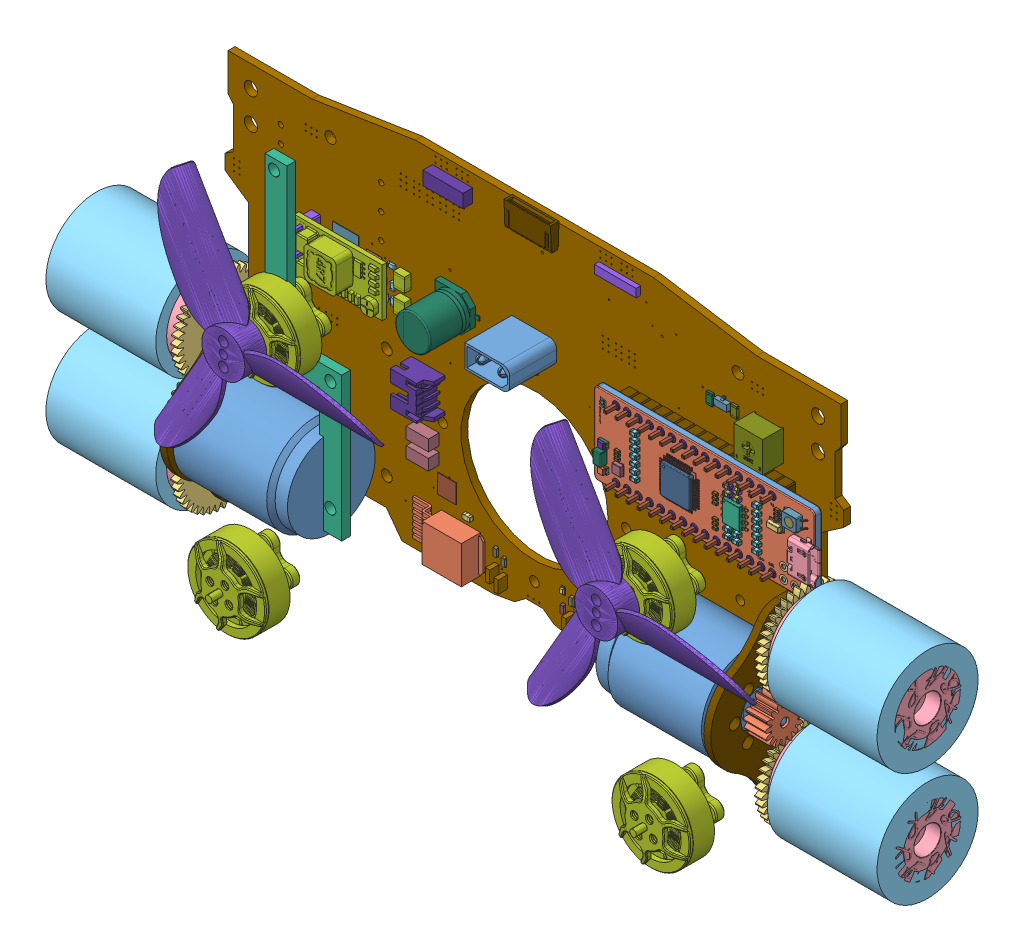
SolidWorks assembly Ensamblaje60, configuration Predeterminado. Lengths in mm.
Overall size (189.47 95.17 43.77).
248 component instances, 80 part files, 7 mates.
Components (placement in the parent):
- placa v11-1: placa v11 [Predeterminado] at (-59.8696 -16.4339 -3.9696) size (140.86 80.97 16.6)
  - placa v11.step-1: placa v11.step [Predeterminado] at origin size (140.86 80.97 16.6)
    - PCB Component.step-1: PCB Component.step [Predeterminado] at origin size (140.86 80.97 16.6)
      - LED-0603 (1).step-1: LED-0603 (1).step [Predeterminado] at (70.275 8.61 1.57) x (0 -1 0) z (0 0 1) size (1.61 0.81 0.61)
        - Pocket002.step-1: Pocket002.step [Predeterminado] at origin size (0.41 0.81 0.21)
        - Pad004.step-1: Pad004.step [Predeterminado] x (1 0 0) z (0 0 -1) size (0.4 0.8 0)
        - Fillet.step-1: Fillet.step [Predeterminado] at origin size (1 0.7 0.4)
        - Pocket001.step-1: Pocket001.step [Predeterminado] at origin size (0.4 0.8 0.2)
        - Pad.step-1: Pad.step [Predeterminado] at origin size (0.8 0.8 0.2)
      - ARDUINO-NANO-3.0.step-1: ARDUINO-NANO-3.0.step [Predeterminado] at (104.204 47.47 1.57) size (51.66 18.54 11.82)
        - 1.step.step-1: 1.step.step [Predeterminado] at (9.2423 0.0433 4.14) x (0 -1 0) z (0 0 1) size (4.9 6 1)
          - 1-0.step.step-1: 1-0.step.step [Predeterminado] at (0 0 0.08) size (4.9 3.9 0.92)
          - 2.step.step-1: 2.step.step [Predeterminado] at (0.635 0 0) size (4.23 6 0.62)
          - Name1.step.step-1: Name1.step.step [Predeterminado] at (-0.0045 -0.5756 0.3787) x (-1 0 0) z (0 1 0) size (0.25 0.13 0.25)
          - thermal pad.step.step-1: thermal pad.step.step [Predeterminado] at (0 0 0.08) x (-1 0 0) z (0 0 -1) size (3.2 2.4 0.1)
        - QFP Template.step.step-1: QFP Template.step.step [Predeterminado] at (-3.3256 -0.4727 4.14) x (0 -1 0) z (0 0 1) size (9 9 1.2)
          - Body.step.step-1: Body.step.step [Predeterminado] at (0 0 0.15) size (7 7 1.05)
          - Leg.step.step-1: Leg.step.step [Predeterminado] at (0 0.25 0) x (1 0 0) z (0 -1 0) size (9 0.75 5.72)
          - Leg.step.step-2: Leg.step.step [Predeterminado] at (-0.25 0 0) x (0 1 0) z (1 0 0) size (9 0.75 5.72)
          - name2.step.step-1: name2.step.step [Predeterminado] at (1.2257 1.5908 1.101) size (0.47 0.47 0.1)
        - QFP Template.step (1).step-1: QFP Template.step (1).step [Predeterminado] at (11.7079 0.2587 2.54) x (0 -1 0) z (0 0 -1) size (9 9 1.2)
          - Body.step.step-1: Body.step.step [Predeterminado] at (0 0 0.15) size (7 7 1.05)
          - Leg.step.step-1: Leg.step.step [Predeterminado] at (0 0.25 0) x (1 0 0) z (0 -1 0) size (9 0.75 5.72)
          - Leg.step.step-2: Leg.step.step [Predeterminado] at (-0.25 0 0) x (0 1 0) z (1 0 0) size (9 0.75 5.72)
          - name2.step.step-1: name2.step.step [Predeterminado] at (1.2257 1.5908 1.101) size (0.47 0.47 0.1)
        - 1-1.step.step-1: 1-1.step.step [Predeterminado] at (-17.0798 -4.3486 4.14) size (2 2 0.8)
          - 1-2.step.step-1: 1-2.step.step [Predeterminado] at (0 0 0.02) size (2 2 0.78)
          - 2-3.step.step-1: 2-3.step.step [Predeterminado] at origin size (2 1.6 0.2)
        - 1-2-4.step.step-1: 1-2-4.step.step [Predeterminado] at (-20.4345 -1.0096 4.14) size (2 1.25 1.09)
          - 1-5.step.step-1: 1-5.step.step [Predeterminado] at (0 0 0.01) size (1.98 1.25 0.58)
          - 2-6.step.step-1: 2-6.step.step [Predeterminado] at (0.001 0 0) size (2 1.25 0.6)
          - 3.step.step-1: 3.step.step [Predeterminado] at (0.001 0 0.59) x (-1 0 0) z (0 0 1) size (1.45 1.25 0.5)
        - 1-3.step.step-1: 1-3.step.step [Predeterminado] at (-20.4345 -6.0538 4.14) size (2 1.25 1.09)
          - 1-7.step.step-1: 1-7.step.step [Predeterminado] at (0 0 0.01) size (1.98 1.25 0.58)
          - 2-8.step.step-1: 2-8.step.step [Predeterminado] at (0.001 0 0) size (2 1.25 0.6)
          - 3-9.step.step-1: 3-9.step.step [Predeterminado] at (0.001 0 0.59) x (-1 0 0) z (0 0 1) size (1.45 1.25 0.5)
        - 1-4.step.step-1: 1-4.step.step [Predeterminado] at (18.758 2.4348 4.14) x (0 -1 0) z (0 0 1) size (2.3 2.86 1.1)
          - 1-10.step.step-1: 1-10.step.step [Predeterminado] at (0 0 0.055) size (1.3 2.86 1.04)
          - 2-11.step.step-1: 2-11.step.step [Predeterminado] x (1 0 0) z (0 -1 0) size (2.3 0.55 2.35)
        - 3-12.step.step-1: 3-12.step.step [Predeterminado] at (14.649 -4.6077 5.09) x (-1 0 0) z (0 0 -1) size (1.6 0.8 0.95)
          - 1-13.step.step-1: 1-13.step.step [Predeterminado] at (-0.78 0.38 0.93) x (1 0 0) z (0 0 -1) size (1.56 0.76 0.91)
          - 2-14.step.step-1: 2-14.step.step [Predeterminado] at (0 0 0.95) x (1 0 0) z (0 0 -1) size (1.6 0.8 0.95)
        - 3-12.step (1).step-1: 3-12.step (1).step [Predeterminado] at (-13.1027 -4.224 5.09) x (-1 0 0) z (0 0 -1) size (1.6 0.8 0.95)
          - 1-13.step.step-1: 1-13.step.step [Predeterminado] at (-0.78 0.38 0.93) x (1 0 0) z (0 0 -1) size (1.56 0.76 0.91)
          - 2-14.step.step-1: 2-14.step.step [Predeterminado] at (0 0 0.95) x (1 0 0) z (0 0 -1) size (1.6 0.8 0.95)
        - 3-12.step (2).step-1: 3-12.step (2).step [Predeterminado] at (14.649 -3.1077 5.09) x (-1 0 0) z (0 0 -1) size (1.6 0.8 0.95)
          - 1-13.step.step-1: 1-13.step.step [Predeterminado] at (-0.78 0.38 0.93) x (1 0 0) z (0 0 -1) size (1.56 0.76 0.91)
          - 2-14.step.step-1: 2-14.step.step [Predeterminado] at (0 0 0.95) x (1 0 0) z (0 0 -1) size (1.6 0.8 0.95)
        - 3-12.step (3).step-1: 3-12.step (3).step [Predeterminado] at (-13.1027 -2.724 5.09) x (-1 0 0) z (0 0 -1) size (1.6 0.8 0.95)
          - 1-13.step.step-1: 1-13.step.step [Predeterminado] at (-0.78 0.38 0.93) x (1 0 0) z (0 0 -1) size (1.56 0.76 0.91)
          - 2-14.step.step-1: 2-14.step.step [Predeterminado] at (0 0 0.95) x (1 0 0) z (0 0 -1) size (1.6 0.8 0.95)
        - 3-12.step (4).step-1: 3-12.step (4).step [Predeterminado] at (14.649 -1.6077 5.09) x (-1 0 0) z (0 0 -1) size (1.6 0.8 0.95)
          - 1-13.step.step-1: 1-13.step.step [Predeterminado] at (-0.78 0.38 0.93) x (1 0 0) z (0 0 -1) size (1.56 0.76 0.91)
          - 2-14.step.step-1: 2-14.step.step [Predeterminado] at (0 0 0.95) x (1 0 0) z (0 0 -1) size (1.6 0.8 0.95)
        - 3-12.step (5).step-1: 3-12.step (5).step [Predeterminado] at (-13.1027 -1.224 5.09) x (-1 0 0) z (0 0 -1) size (1.6 0.8 0.95)
          - 1-13.step.step-1: 1-13.step.step [Predeterminado] at (-0.78 0.38 0.93) x (1 0 0) z (0 0 -1) size (1.56 0.76 0.91)
          - 2-14.step.step-1: 2-14.step.step [Predeterminado] at (0 0 0.95) x (1 0 0) z (0 0 -1) size (1.6 0.8 0.95)
        - 3-12.step (6).step-1: 3-12.step (6).step [Predeterminado] at (14.649 -0.1077 5.09) x (-1 0 0) z (0 0 -1) size (1.6 0.8 0.95)
          - 1-13.step.step-1: 1-13.step.step [Predeterminado] at (-0.78 0.38 0.93) x (1 0 0) z (0 0 -1) size (1.56 0.76 0.91)
          - 2-14.step.step-1: 2-14.step.step [Predeterminado] at (0 0 0.95) x (1 0 0) z (0 0 -1) size (1.6 0.8 0.95)
        - 3-12.step (7).step-1: 3-12.step (7).step [Predeterminado] at (-13.1027 0.276 5.09) x (-1 0 0) z (0 0 -1) size (1.6 0.8 0.95)
          - 1-13.step.step-1: 1-13.step.step [Predeterminado] at (-0.78 0.38 0.93) x (1 0 0) z (0 0 -1) size (1.56 0.76 0.91)
          - 2-14.step.step-1: 2-14.step.step [Predeterminado] at (0 0 0.95) x (1 0 0) z (0 0 -1) size (1.6 0.8 0.95)
        - 3-12.step (8).step-1: 3-12.step (8).step [Predeterminado] at (14.649 1.3923 5.09) x (-1 0 0) z (0 0 -1) size (1.6 0.8 0.95)
          - 1-13.step.step-1: 1-13.step.step [Predeterminado] at (-0.78 0.38 0.93) x (1 0 0) z (0 0 -1) size (1.56 0.76 0.91)
          - 2-14.step.step-1: 2-14.step.step [Predeterminado] at (0 0 0.95) x (1 0 0) z (0 0 -1) size (1.6 0.8 0.95)
        - 3-12.step (9).step-1: 3-12.step (9).step [Predeterminado] at (-13.1027 1.776 5.09) x (-1 0 0) z (0 0 -1) size (1.6 0.8 0.95)
          - 1-13.step.step-1: 1-13.step.step [Predeterminado] at (-0.78 0.38 0.93) x (1 0 0) z (0 0 -1) size (1.56 0.76 0.91)
          - 2-14.step.step-1: 2-14.step.step [Predeterminado] at (0 0 0.95) x (1 0 0) z (0 0 -1) size (1.6 0.8 0.95)
        - 3-12.step (10).step-1: 3-12.step (10).step [Predeterminado] at (14.649 2.8923 5.09) x (-1 0 0) z (0 0 -1) size (1.6 0.8 0.95)
          - 1-13.step.step-1: 1-13.step.step [Predeterminado] at (-0.78 0.38 0.93) x (1 0 0) z (0 0 -1) size (1.56 0.76 0.91)
          - 2-14.step.step-1: 2-14.step.step [Predeterminado] at (0 0 0.95) x (1 0 0) z (0 0 -1) size (1.6 0.8 0.95)
        - 3-12.step (11).step-1: 3-12.step (11).step [Predeterminado] at (-13.1027 3.276 5.09) x (-1 0 0) z (0 0 -1) size (1.6 0.8 0.95)
          - 1-13.step.step-1: 1-13.step.step [Predeterminado] at (-0.78 0.38 0.93) x (1 0 0) z (0 0 -1) size (1.56 0.76 0.91)
          - 2-14.step.step-1: 2-14.step.step [Predeterminado] at (0 0 0.95) x (1 0 0) z (0 0 -1) size (1.6 0.8 0.95)
        - 3-12.step (12).step-1: 3-12.step (12).step [Predeterminado] at (14.649 4.3923 5.09) x (-1 0 0) z (0 0 -1) size (1.6 0.8 0.95)
          - 1-13.step.step-1: 1-13.step.step [Predeterminado] at (-0.78 0.38 0.93) x (1 0 0) z (0 0 -1) size (1.56 0.76 0.91)
          - 2-14.step.step-1: 2-14.step.step [Predeterminado] at (0 0 0.95) x (1 0 0) z (0 0 -1) size (1.6 0.8 0.95)
        - 3-12.step (13).step-1: 3-12.step (13).step [Predeterminado] at (-13.1027 4.776 5.09) x (-1 0 0) z (0 0 -1) size (1.6 0.8 0.95)
          - 1-13.step.step-1: 1-13.step.step [Predeterminado] at (-0.78 0.38 0.93) x (1 0 0) z (0 0 -1) size (1.56 0.76 0.91)
          - 2-14.step.step-1: 2-14.step.step [Predeterminado] at (0 0 0.95) x (1 0 0) z (0 0 -1) size (1.6 0.8 0.95)
        - 3-12.step (14).step-1: 3-12.step (14).step [Predeterminado] at (10.1169 -4.9732 4.14) size (1.6 0.8 0.95)
          - 1-13.step.step-1: 1-13.step.step [Predeterminado] at (-0.78 0.38 0.93) x (1 0 0) z (0 0 -1) size (1.56 0.76 0.91)
          - 2-14.step.step-1: 2-14.step.step [Predeterminado] at (0 0 0.95) x (1 0 0) z (0 0 -1) size (1.6 0.8 0.95)
        - 3-12.step (15).step-1: 3-12.step (15).step [Predeterminado] at (8.1169 -4.9732 4.14) size (1.6 0.8 0.95)
          - 1-13.step.step-1: 1-13.step.step [Predeterminado] at (-0.78 0.38 0.93) x (1 0 0) z (0 0 -1) size (1.56 0.76 0.91)
          - 2-14.step.step-1: 2-14.step.step [Predeterminado] at (0 0 0.95) x (1 0 0) z (0 0 -1) size (1.6 0.8 0.95)
        - 3-12.step (16).step-1: 3-12.step (16).step [Predeterminado] at (10.1169 -3.4732 4.14) size (1.6 0.8 0.95)
          - 1-13.step.step-1: 1-13.step.step [Predeterminado] at (-0.78 0.38 0.93) x (1 0 0) z (0 0 -1) size (1.56 0.76 0.91)
          - 2-14.step.step-1: 2-14.step.step [Predeterminado] at (0 0 0.95) x (1 0 0) z (0 0 -1) size (1.6 0.8 0.95)
        - 3-12.step (17).step-1: 3-12.step (17).step [Predeterminado] at (8.1169 -3.4732 4.14) size (1.6 0.8 0.95)
          - 1-13.step.step-1: 1-13.step.step [Predeterminado] at (-0.78 0.38 0.93) x (1 0 0) z (0 0 -1) size (1.56 0.76 0.91)
          - 2-14.step.step-1: 2-14.step.step [Predeterminado] at (0 0 0.95) x (1 0 0) z (0 0 -1) size (1.6 0.8 0.95)
        - 3_MIR.step.step-1: 3_MIR.step.step [Predeterminado] at (10.1169 4.9732 4.14) x (1 0 0) z (0 0 -1) size (1.6 0.8 0.95)
          - 1_MIR.step.step-1: 1_MIR.step.step [Predeterminado] at (-0.78 0.38 -0.93) x (1 0 0) z (0 0 -1) size (1.56 0.76 0.91)
          - 2_MIR.step.step-1: 2_MIR.step.step [Predeterminado] at (0 0 -0.95) x (1 0 0) z (0 0 -1) size (1.6 0.8 0.95)
        - 3_MIR.step (1).step-1: 3_MIR.step (1).step [Predeterminado] at (8.1169 4.9732 4.14) x (1 0 0) z (0 0 -1) size (1.6 0.8 0.95)
          - 1_MIR.step.step-1: 1_MIR.step.step [Predeterminado] at (-0.78 0.38 -0.93) x (1 0 0) z (0 0 -1) size (1.56 0.76 0.91)
          - 2_MIR.step.step-1: 2_MIR.step.step [Predeterminado] at (0 0 -0.95) x (1 0 0) z (0 0 -1) size (1.6 0.8 0.95)
        - 3_MIR.step (2).step-1: 3_MIR.step (2).step [Predeterminado] at (10.1169 3.4732 4.14) x (1 0 0) z (0 0 -1) size (1.6 0.8 0.95)
          - 1_MIR.step.step-1: 1_MIR.step.step [Predeterminado] at (-0.78 0.38 -0.93) x (1 0 0) z (0 0 -1) size (1.56 0.76 0.91)
          - 2_MIR.step.step-1: 2_MIR.step.step [Predeterminado] at (0 0 -0.95) x (1 0 0) z (0 0 -1) size (1.6 0.8 0.95)
        - 3_MIR.step (3).step-1: 3_MIR.step (3).step [Predeterminado] at (8.1169 3.4732 4.14) x (1 0 0) z (0 0 -1) size (1.6 0.8 0.95)
          - 1_MIR.step.step-1: 1_MIR.step.step [Predeterminado] at (-0.78 0.38 -0.93) x (1 0 0) z (0 0 -1) size (1.56 0.76 0.91)
          - 2_MIR.step.step-1: 2_MIR.step.step [Predeterminado] at (0 0 -0.95) x (1 0 0) z (0 0 -1) size (1.6 0.8 0.95)
        - 3-1.step.step-1: 3-1.step.step [Predeterminado] at (19.0751 5.5632 4.69) x (-1 0 0) z (0 0 -1) size (1 0.5 0.55)
          - 1-15.step.step-1: 1-15.step.step [Predeterminado] at (-0.49 0.24 0.54) x (1 0 0) z (0 0 -1) size (0.98 0.48 0.53)
          - 2-16.step.step-1: 2-16.step.step [Predeterminado] at (-0.5 0.25 0.55) x (1 0 0) z (0 0 -1) size (1 0.5 0.55)
        - 3-1.step (1).step-1: 3-1.step (1).step [Predeterminado] at (19.0751 4.7491 4.69) x (-1 0 0) z (0 0 -1) size (1 0.5 0.55)
          - 1-15.step.step-1: 1-15.step.step [Predeterminado] at (-0.49 0.24 0.54) x (1 0 0) z (0 0 -1) size (0.98 0.48 0.53)
          - 2-16.step.step-1: 2-16.step.step [Predeterminado] at (-0.5 0.25 0.55) x (1 0 0) z (0 0 -1) size (1 0.5 0.55)
        - 3-1.step (2).step-1: 3-1.step (2).step [Predeterminado] at (19.0751 3.9392 4.69) x (-1 0 0) z (0 0 -1) size (1 0.5 0.55)
          - 1-15.step.step-1: 1-15.step.step [Predeterminado] at (-0.49 0.24 0.54) x (1 0 0) z (0 0 -1) size (0.98 0.48 0.53)
          - 2-16.step.step-1: 2-16.step.step [Predeterminado] at (-0.5 0.25 0.55) x (1 0 0) z (0 0 -1) size (1 0.5 0.55)
        - 3-1.step (3).step-1: 3-1.step (3).step [Predeterminado] at (-17.3312 -0.9835 4.69) x (-1 0 0) z (0 0 -1) size (1 0.5 0.55)
          - 1-15.step.step-1: 1-15.step.step [Predeterminado] at (-0.49 0.24 0.54) x (1 0 0) z (0 0 -1) size (0.98 0.48 0.53)
          - 2-16.step.step-1: 2-16.step.step [Predeterminado] at (-0.5 0.25 0.55) x (1 0 0) z (0 0 -1) size (1 0.5 0.55)
        - 3-1.step (4).step-1: 3-1.step (4).step [Predeterminado] at (-17.3312 -2.5605 4.69) x (-1 0 0) z (0 0 -1) size (1 0.5 0.55)
          - 1-15.step.step-1: 1-15.step.step [Predeterminado] at (-0.49 0.24 0.54) x (1 0 0) z (0 0 -1) size (0.98 0.48 0.53)
          - 2-16.step.step-1: 2-16.step.step [Predeterminado] at (-0.5 0.25 0.55) x (1 0 0) z (0 0 -1) size (1 0.5 0.55)
        - 3-1.step (5).step-1: 3-1.step (5).step [Predeterminado] at (-17.3312 -1.7295 4.69) x (-1 0 0) z (0 0 -1) size (1 0.5 0.55)
          - 1-15.step.step-1: 1-15.step.step [Predeterminado] at (-0.49 0.24 0.54) x (1 0 0) z (0 0 -1) size (0.98 0.48 0.53)
          - 2-16.step.step-1: 2-16.step.step [Predeterminado] at (-0.5 0.25 0.55) x (1 0 0) z (0 0 -1) size (1 0.5 0.55)
        - 3-1.step (6).step-1: 3-1.step (6).step [Predeterminado] at (5.0242 -5.0165 4.69) x (-1 0 0) z (0 0 -1) size (1 0.5 0.55)
          - 1-15.step.step-1: 1-15.step.step [Predeterminado] at (-0.49 0.24 0.54) x (1 0 0) z (0 0 -1) size (0.98 0.48 0.53)
          - 2-16.step.step-1: 2-16.step.step [Predeterminado] at (-0.5 0.25 0.55) x (1 0 0) z (0 0 -1) size (1 0.5 0.55)
        - 3-1.step (7).step-1: 3-1.step (7).step [Predeterminado] at (5.0242 -4.0978 4.69) x (-1 0 0) z (0 0 -1) size (1 0.5 0.55)
          - 1-15.step.step-1: 1-15.step.step [Predeterminado] at (-0.49 0.24 0.54) x (1 0 0) z (0 0 -1) size (0.98 0.48 0.53)
          - 2-16.step.step-1: 2-16.step.step [Predeterminado] at (-0.5 0.25 0.55) x (1 0 0) z (0 0 -1) size (1 0.5 0.55)
        - 3-1.step (8).step-1: 3-1.step (8).step [Predeterminado] at (5.0242 -3.2174 4.69) x (-1 0 0) z (0 0 -1) size (1 0.5 0.55)
          - 1-15.step.step-1: 1-15.step.step [Predeterminado] at (-0.49 0.24 0.54) x (1 0 0) z (0 0 -1) size (0.98 0.48 0.53)
          - 2-16.step.step-1: 2-16.step.step [Predeterminado] at (-0.5 0.25 0.55) x (1 0 0) z (0 0 -1) size (1 0.5 0.55)
        - 3-1.step (9).step-1: 3-1.step (9).step [Predeterminado] at (5.0242 -0.0165 4.69) x (-1 0 0) z (0 0 -1) size (1 0.5 0.55)
          - 1-15.step.step-1: 1-15.step.step [Predeterminado] at (-0.49 0.24 0.54) x (1 0 0) z (0 0 -1) size (0.98 0.48 0.53)
          - 2-16.step.step-1: 2-16.step.step [Predeterminado] at (-0.5 0.25 0.55) x (1 0 0) z (0 0 -1) size (1 0.5 0.55)
        - 3-1.step (10).step-1: 3-1.step (10).step [Predeterminado] at (5.0242 0.9022 4.69) x (-1 0 0) z (0 0 -1) size (1 0.5 0.55)
          - 1-15.step.step-1: 1-15.step.step [Predeterminado] at (-0.49 0.24 0.54) x (1 0 0) z (0 0 -1) size (0.98 0.48 0.53)
          - 2-16.step.step-1: 2-16.step.step [Predeterminado] at (-0.5 0.25 0.55) x (1 0 0) z (0 0 -1) size (1 0.5 0.55)
        - 3-1.step (11).step-1: 3-1.step (11).step [Predeterminado] at (5.0242 1.7826 4.69) x (-1 0 0) z (0 0 -1) size (1 0.5 0.55)
          - 1-15.step.step-1: 1-15.step.step [Predeterminado] at (-0.49 0.24 0.54) x (1 0 0) z (0 0 -1) size (0.98 0.48 0.53)
          - 2-16.step.step-1: 2-16.step.step [Predeterminado] at (-0.5 0.25 0.55) x (1 0 0) z (0 0 -1) size (1 0.5 0.55)
        - 1-17.step.step-1: 1-17.step.step [Predeterminado] at (2.2426 0 2.54) x (0 -1 0) z (0 0 1) size (15.88 36.2 11.76)
        - 2-18.step.step-1: 2-18.step.step [Predeterminado] at (2.2426 0 2.54) x (0 -1 0) z (0 0 1) size (1.95 1.95 0.2)
        - 3-19.step.step-1: 3-19.step.step [Predeterminado] at (2.2426 0 2.54) x (0 -1 0) z (0 0 1) size (1.8 5.28 0.86)
        - 4.step.step-1: 4.step.step [Predeterminado] at (2.2426 0 2.54) x (0 -1 0) z (0 0 1) size (2.98 3.39 1.49)
        - 6.step.step-1: 6.step.step [Predeterminado] at (2.2426 0 2.54) x (0 -1 0) z (0 0 1) size (2.83 1.84 1.5)
        - 7.step.step-1: 7.step.step [Predeterminado] at (2.2426 0 2.54) x (0 -1 0) z (0 0 1) size (0.97 0.6 0.51)
        - 8.step.step-1: 8.step.step [Predeterminado] at (2.2426 0 2.54) x (0 -1 0) z (0 0 1) size (16.96 37.28 0.1)
        - 9.step.step-1: 9.step.step [Predeterminado] at (2.2426 0 2.54) x (0 -1 0) z (0 0 1) size (17.78 38.1 2.54)
        - 10.step.step-1: 10.step.step [Predeterminado] at (2.2426 0 2.54) x (0 -1 0) z (0 0 1) size (18.54 50.29 1.2)
        - 11.step.step-1: 11.step.step [Predeterminado] at (2.2426 0 2.54) x (0 -1 0) z (0 0 1) size (18.54 50.29 1.6)
        - 12.step.step-1: 12.step.step [Predeterminado] at (2.2426 0 2.54) x (0 -1 0) z (0 0 1) size (4.34 6.88 1.6)
        - USB Connector.step.step-1: USB Connector.step.step [Predeterminado] at (26.0074 -0.1867 5.365) x (0 1 0) z (1 0 0) size (8.2 3.3 5.4)
        - 13.step.step-1: 13.step.step [Predeterminado] at (2.2426 0 4.14) x (0 -1 0) z (0 0 1) size (12.46 38.74 0)
        - STM Logo.step.step-1: STM Logo.step.step [Predeterminado] at (-19.8495 -2.5718 4.041) x (0 -1 0) z (0 0 1) size (5.5 1.52 0.1)
      - HW-613.step-1: HW-613.step [Predeterminado] at (12.49 44.591 1.57) size (20 11 13.1)
        - 05KJ_Mini_PCB_Regulator.step-1: 05KJ_Mini_PCB_Regulator.step [Predeterminado] at (19.8629 10.8309 2.3992) x (0 -1 0) z (-1 0 0) size (11 4.81 20)
        - 1_Male_Pin_2.54_mm.step-1: 1_Male_Pin_2.54_mm.step [Predeterminado] at (1.6879 8.8159 5.3992) x (0 1 0) z (-1 0 0) size (2.54 11.1 2.4)
        - 1_Male_Pin_2.54_mm.step-2: 1_Male_Pin_2.54_mm.step [Predeterminado] at (1.6879 6.2759 5.3992) x (0 1 0) z (-1 0 0) size (2.54 11.1 2.4)
        - 1_Male_Pin_2.54_mm.step-3: 1_Male_Pin_2.54_mm.step [Predeterminado] at (1.6879 3.7359 5.3992) x (0 1 0) z (-1 0 0) size (2.54 11.1 2.4)
        - 1_Male_Pin_2.54_mm.step-4: 1_Male_Pin_2.54_mm.step [Predeterminado] at (1.6879 1.1959 5.3992) x (0 1 0) z (-1 0 0) size (2.54 11.1 2.4)
      - Board.step-1: Board.step [Predeterminado] at origin size (140.86 80.59 1.57)
      - MOMENTARY-SWITCH-SPST-SMD-5.2-REDUNDANT.step-1: MOMENTARY-SWITCH-SPST-SMD-5.2-REDUNDANT.step [Predeterminado] at (7.486 44.336 1.57) size (6.4 5.3 1.5)
      - 10k_2.step-1: 10k_2.step [Predeterminado] at (7.386 40.707 1.57) size (2.5 1.4 0.5)
      - LED-0603.step-1: LED-0603.step [Predeterminado] at (55.035 8.61 1.57) x (0 -1 0) z (0 0 1) size (2.1 0.8 0.6)
      - 10k.step-1: 10k.step [Predeterminado] at (70.312 4.989 1.57) x (0 -1 0) z (0 0 1) size (2.1 0.8 0.6)
      - 2N7002CK.step-1: 2N7002CK.step [Predeterminado] at (106.952 63.962 1.57) size (3 2.5 1.1)
      - 103.step-1: 103.step [Predeterminado] at (103.896 63.305 1.57) x (0 -1 0) z (0 0 1) size (2.5 1.4 0.5)
      - 10k_1.step-1: 10k_1.step [Predeterminado] at (109.485 63.628 1.57) x (0 -1 0) z (0 0 1) size (2.5 1.4 0.5)
      - JST-XH-03-PIN-LONG-PAD.step-1: JST-XH-03-PIN-LONG-PAD.step [Predeterminado] at (39.428 34.17 1.57) x (0 -1 0) z (0 0 1) size (7.9 7.6 8.2)
      - FH12-08S-1SH.step-1: FH12-08S-1SH.step [Predeterminado] at (63.91 77.561 1.57) x (-1 0 0) z (0 0 1) size (10.6 6.5 1.92)
      - 10k_2.step-2: 10k_2.step [Predeterminado] at (7.262 48.989 1.57) size (2.5 1.4 0.5)
      - LED-0603.step-2: LED-0603.step [Predeterminado] at (56.895 7.53 1.57) x (0 -1 0) z (0 0 1) size (2.1 0.8 0.6)
      - LED-0603.step-3: LED-0603.step [Predeterminado] at (72.322 7.486 1.57) x (0 -1 0) z (0 0 1) size (2.1 0.8 0.6)
      - XT30UPB-M.step-1: XT30UPB-M.step [Predeterminado] at (63.686 54.256 1.57) x (-1 0 0) z (0 0 1) size (10.2 5.25 13.7)
      - TLE5206-2G.step-1: TLE5206-2G.step [Predeterminado] at (44.309 6.214 1.57) x (0 -1 0) z (0 0 1) size (8.52 16 4.4)
      - CAPC1608X85.step-1: CAPC1608X85.step [Predeterminado] at (79.287 12.679 1.57) x (-1 0 0) z (0 0 1) size (1.75 0.95 0.85)
      - CAPC1608X85.step-2: CAPC1608X85.step [Predeterminado] at (48.839 12.459 1.57) x (-1 0 0) z (0 0 1) size (1.75 0.95 0.85)
      - MP2315GJ.step-1: MP2315GJ.step [Predeterminado] at (26.969 52.158 1.57) x (-1 0 0) z (0 0 1) size (3.46 2.1 0.1)
      - 200k.step-1: 200k.step [Predeterminado] at (27.103 47.618 1.57) size (1.6 0.86 0.51)
      - 200k.step-2: 200k.step [Predeterminado] at (29.997 46.286 1.57) x (0 1 0) z (0 0 1) size (1.6 0.86 0.51)
      - 200k.step-3: 200k.step [Predeterminado] at (24.743 45.644 1.57) size (1.6 0.86 0.51)
      - 200k.step-4: 200k.step [Predeterminado] at (31.702 46.341 1.57) x (0 -1 0) z (0 0 1) size (1.6 0.86 0.51)
      - 200k.step-5: 200k.step [Predeterminado] at (31.645 49.39 1.57) x (0 1 0) z (0 0 1) size (1.6 0.86 0.51)
      - 200k.step-6: 200k.step [Predeterminado] at (31.3 53.202 1.57) size (1.6 0.86 0.51)
      - 22uf.step-1: 22uf.step [Predeterminado] at (23.406 47.636 1.57) size (1.6 0.86 0.86)
      - 22uf.step-2: 22uf.step [Predeterminado] at (27.652 45.634 1.57) size (1.6 0.86 0.86)
      - 22uf.step-3: 22uf.step [Predeterminado] at (18.728 45.514 1.57) size (1.6 0.86 0.86)
      - 22uf.step-4: 22uf.step [Predeterminado] at (21.82 45.634 1.57) x (-1 0 0) z (0 0 1) size (1.6 0.86 0.86)
      - 22uf.step-5: 22uf.step [Predeterminado] at (29.634 49.37 1.57) x (0 1 0) z (0 0 1) size (1.6 0.86 0.86)
      - 22uf.step-6: 22uf.step [Predeterminado] at (18.755 47.622 1.57) size (1.6 0.86 0.86)
      - C1210.step-1: C1210.step [Predeterminado] at (34.29 52.07 1.57) x (0 -1 0) z (0 0 1) size (3.2 2.5 1.55)
      - C1210.step-2: C1210.step [Predeterminado] at (34.29 46.99 1.57) x (0 1 0) z (0 0 1) size (3.2 2.5 1.55)
      - 1X04.step-1: 1X04.step [Predeterminado] at (79.26 76.438 1.57) size (9.5 1.88 1.05)
      - 10k_3.step-1: 10k_3.step [Predeterminado] at (55.035 4.8 1.57) x (0 -1 0) z (0 0 1) size (2.8 1 2.1)
      - 10k_3.step-2: 10k_3.step [Predeterminado] at (92.194 65.647 0) x (0 1 0) z (0 0 -1) size (2.8 1 2.1)
      - 10k_3.step-3: 10k_3.step [Predeterminado] at (35.601 12.641 0) x (0 -1 0) z (0 0 -1) size (2.8 1 2.1)
      - 10k_3.step-4: 10k_3.step [Predeterminado] at (47.48 65.436 0) x (0 1 0) z (0 0 -1) size (2.8 1 2.1)
      - 10k_3.step-5: 10k_3.step [Predeterminado] at (82.596 12.429 0) x (0 -1 0) z (0 0 -1) size (2.8 1 2.1)
      - 10k_3.step-6: 10k_3.step [Predeterminado] at (56.965 3.798 1.57) x (0 1 0) z (0 0 1) size (2.8 1 2.1)
      - 10k_3.step-7: 10k_3.step [Predeterminado] at (72.365 3.894 1.57) x (0 -1 0) z (0 0 1) size (2.8 1 2.1)
      - LED-0603 (2).step-1: LED-0603 (2).step [Predeterminado] at (86.133 65.321 0) x (1 0 0) z (0 0 -1) size (2.75 1 1.86)
      - LED-0603 (2).step-2: LED-0603 (2).step [Predeterminado] at (41.633 11.485 0) x (1 0 0) z (0 0 -1) size (2.75 1 1.86)
      - LED-0603 (2).step-3: LED-0603 (2).step [Predeterminado] at (41.68 65.48 0) x (1 0 0) z (0 0 -1) size (2.75 1 1.86)
      - LED-0603 (2).step-4: LED-0603 (2).step [Predeterminado] at (85.968 11.242 0) x (1 0 0) z (0 0 -1) size (2.75 1 1.86)
      - LED-0603 (2).step-5: LED-0603 (2).step [Predeterminado] at (7.24 50.476 1.57) size (2.75 1 1.86)
      - 153CLV-0405.step-1: 153CLV-0405.step [Predeterminado] at (43.742 15.388 1.57) x (-1 0 0) z (0 0 1) size (4.3 4.3 0.1)
      - 153CLV-0405.step-2: 153CLV-0405.step [Predeterminado] at (83.228 15.388 1.57) x (-1 0 0) z (0 0 1) size (4.3 4.3 0.1)
      - TLE5206-2G_1.step-1: TLE5206-2G_1.step [Predeterminado] at (84.077 6.486 1.57) x (0 1 0) z (0 0 1) size (8.52 16 4.4)
      - SMD2,54-5,08.step-1: SMD2,54-5,08.step [Predeterminado] at (39.37 24.13 1.57) x (0 1 0) z (0 0 1) size (2.54 5.08 2.44)
      - SMD2,54-5,08.step-2: SMD2,54-5,08.step [Predeterminado] at (39.37 20.32 1.57) x (0 1 0) z (0 0 1) size (2.54 5.08 2.44)
      - SMD2,54-5,08.step-3: SMD2,54-5,08.step [Predeterminado] at (87.63 24.13 1.57) x (0 1 0) z (0 0 1) size (2.54 5.08 2.44)
      - SMD2,54-5,08.step-4: SMD2,54-5,08.step [Predeterminado] at (87.63 20.32 1.57) x (0 1 0) z (0 0 1) size (2.54 5.08 2.44)
      - 4.2uh.step-1: 4.2uh.step [Predeterminado] at (20.701 52.121 1.57) x (-1 0 0) z (0 0 1) size (6 6 0.1)
      - 153CLV-0807.step-1: 153CLV-0807.step [Predeterminado] at (46.349 52.61 1.57) size (9.8 8 10.51)
      - B25P.step-1: B25P.step [Predeterminado] at (117 62 1.57) size (6.61 7.21 6.73)
      - MA04-1.step-1: MA04-1.step [Predeterminado] at (44.979 76.037 1.57) size (9.14 3.05 2.19)
- Ensamblaje 40t-2: Ensamblaje 40t [Predeterminado] at (27.1044 5.1482 10.0162) x (0 1 0) z (1 0 0) size (53.09 31.11 59.6)
  - SOPORTE PARA 40T-1: SOPORTE PARA 40T [Predeterminado] at (-2.7975 -1.3158 37.7691) size (37.5 22.58 1.6)
  - motor-1: motor [Predeterminado] at (-2.7975 -1.3158 11.7691) x (0 0 1) z (-0.999998 -0.002002 0) size (33 22 22)
  - 16T-1: 16T [Predeterminado] at (-2.7975 -1.3158 39.7691) x (0.903123 0.429382 0) z (0 0 1) size (8.96 8.96 5)
  - 40T-1: 40T [Predeterminado] at (-15.7975 -7.3158 42.3691) x (0.369504 0.929229 0) z (0.929229 -0.369504 0) size (20.99 1.5 20.99)
  - 40T-2: 40T [Predeterminado] at (10.2025 -7.3158 42.3691) x (0.135333 0.9908 0) z (0.9908 -0.135333 0) size (20.99 1.5 20.99)
  - rin-1: rin [Predeterminado] at (10.2025 -7.3158 46.3691) x (0.124373 -0.992236 0) z (0 0 1) size (18 18 27.5)
  - llanta-1: llanta [Predeterminado] at (10.2025 -7.3158 46.2691) x (0.189107 0.981956 0) z (0.981956 -0.189107 0) size (23 25 23)
  - rin-2: rin [Predeterminado] at (-15.7975 -7.3158 46.3691) x (0.124373 -0.992236 0) z (0 0 1) size (18 18 27.5)
  - llanta-2: llanta [Predeterminado] at (-15.7975 -7.3158 46.2691) x (0.189107 0.981956 0) z (0.981956 -0.189107 0) size (23 25 23)
- Ensamblaje 40t-3: Ensamblaje 40t [Predeterminado] at (-19.6285 -4.7323 10.0162) x (0 -1 0) z (-1 0 0) size (53.09 31.11 59.6)
  - SOPORTE PARA 40T-1: SOPORTE PARA 40T [Predeterminado] at (-2.7975 -1.3158 37.7691) size (37.5 22.58 1.6)
  - motor-1: motor [Predeterminado] at (-2.7975 -1.3158 11.7691) x (0 0 1) z (-0.999998 -0.002002 0) size (33 22 22)
  - 16T-1: 16T [Predeterminado] at (-2.7975 -1.3158 39.7691) x (0.903123 0.429382 0) z (0 0 1) size (8.96 8.96 5)
  - 40T-1: 40T [Predeterminado] at (-15.7975 -7.3158 42.3691) x (0.369504 0.929229 0) z (0.929229 -0.369504 0) size (20.99 1.5 20.99)
  - 40T-2: 40T [Predeterminado] at (10.2025 -7.3158 42.3691) x (0.135333 0.9908 0) z (0.9908 -0.135333 0) size (20.99 1.5 20.99)
  - rin-1: rin [Predeterminado] at (10.2025 -7.3158 46.3691) x (0.124373 -0.992236 0) z (0 0 1) size (18 18 27.5)
  - llanta-1: llanta [Predeterminado] at (10.2025 -7.3158 46.2691) x (0.189107 0.981956 0) z (0.981956 -0.189107 0) size (23 25 23)
  - rin-2: rin [Predeterminado] at (-15.7975 -7.3158 46.3691) x (0.124373 -0.992236 0) z (0 0 1) size (18 18 27.5)
  - llanta-2: llanta [Predeterminado] at (-15.7975 -7.3158 46.2691) x (0.189107 0.981956 0) z (0.981956 -0.189107 0) size (23 25 23)
- frame-1: frame [Predeterminado] at (-59.8602 15.0313 8.4484) x (1 0 0) z (0 -1 0) size (29.2 2 67.75)
- 1404 motor.step-1: 1404 motor.step [Predeterminado] at (53.5446 -20.5527 10.4484) size (17.9 17.9 14.55)
  - 1404 motor_1.step-1: 1404 motor_1.step [Predeterminado] at origin size (17.9 17.9 14.55)
- 1404 motor.step-2: 1404 motor.step [Predeterminado] at (-42.2062 -21.845 11.3394) size (17.9 17.9 14.55)
  - 1404 motor_1.step-1: 1404 motor_1.step [Predeterminado] at origin size (17.9 17.9 14.55)
- 1404 motor.step-3: 1404 motor.step [Predeterminado] at (53.1149 26.1877 14.2365) size (17.9 17.9 14.55)
  - 1404 motor_1.step-1: 1404 motor_1.step [Predeterminado] at origin size (17.9 17.9 14.55)
- 1404 motor.step-4: 1404 motor.step [Predeterminado] at (-41.0148 25.4579 5.2964) size (17.9 17.9 14.55)
  - 1404 motor_1.step-1: 1404 motor_1.step [Predeterminado] at origin size (17.9 17.9 14.55)
- RHR-25_tri_V5_CCW-1: RHR-25_tri_V5_CCW [Predeterminado] at (-166.061 -109.0647 18.3912) size (51.66 56.49 5.3)
- RHR-25_tri_V5_CCW-2: RHR-25_tri_V5_CCW [Predeterminado] at (-71.9877 -108.4233 27.5464) size (51.66 56.49 5.3)
Mates (geometry in assembly coordinates):
- Coincidente1: coincident anti-aligned: plane of placa v11-1/placa v11.step-1/PCB Component.step-1/Board.step-1 through (3.7379 23.7056 -2.3996) normal (0 0 1); plane of Ensamblaje 40t-3/SOPORTE PARA 40T-1 through (-58.9976 -1.9347 -2.3996) normal (0 0 -1)
- Coincidente2: coincident aligned: plane of placa v11-1/placa v11.step-1/PCB Component.step-1/Board.step-1 through (-58.9976 17.1531 -3.9696) normal (-1 0 0); plane of Ensamblaje 40t-3/SOPORTE PARA 40T-1 through (-58.9976 -1.9347 8.7004) normal (-1 0 0)
- Coincidente3: coincident aligned: plane of placa v11-1/placa v11.step-1/PCB Component.step-1/Board.step-1 through (66.4734 -13.2269 -3.9696) normal (1 0 0); plane of Ensamblaje 40t-2/SOPORTE PARA 40T-1 through (66.4734 2.3507 8.7004) normal (1 0 0)
- Coincidente4: coincident anti-aligned: plane of placa v11-1/placa v11.step-1/PCB Component.step-1/Board.step-1 through (3.7379 23.7056 -2.3996) normal (0 0 1); plane of Ensamblaje 40t-2/SOPORTE PARA 40T-1 through (66.4734 2.3507 -2.3996) normal (0 0 -1)
- Concéntrica2: concentric aligned: cylinder of placa v11-1/placa v11.step-1/PCB Component.step-1/Board.step-1 through (-42.7016 54.8511 -3.9696) axis (0 0 1) radius 1.25; cylinder of frame-1 through (-42.7016 54.8511 8.4484) axis (0 0 1) radius 1.25
- Concéntrica3: concentric aligned: cylinder of placa v11-1/placa v11.step-1/PCB Component.step-1/Board.step-1 through (-29.8716 19.5671 -3.9696) axis (0 0 1) radius 1.25; cylinder of frame-1 through (-29.8716 19.5671 8.4484) axis (0 0 1) radius 1.25
- Coincidente5: coincident anti-aligned: plane of frame-1 through (-59.8602 15.0313 10.4484) normal (0 0 1); plane of 1404 motor.step-1/1404 motor_1.step-1 through (53.5446 -20.5527 10.4484) normal (0 0 -1)
